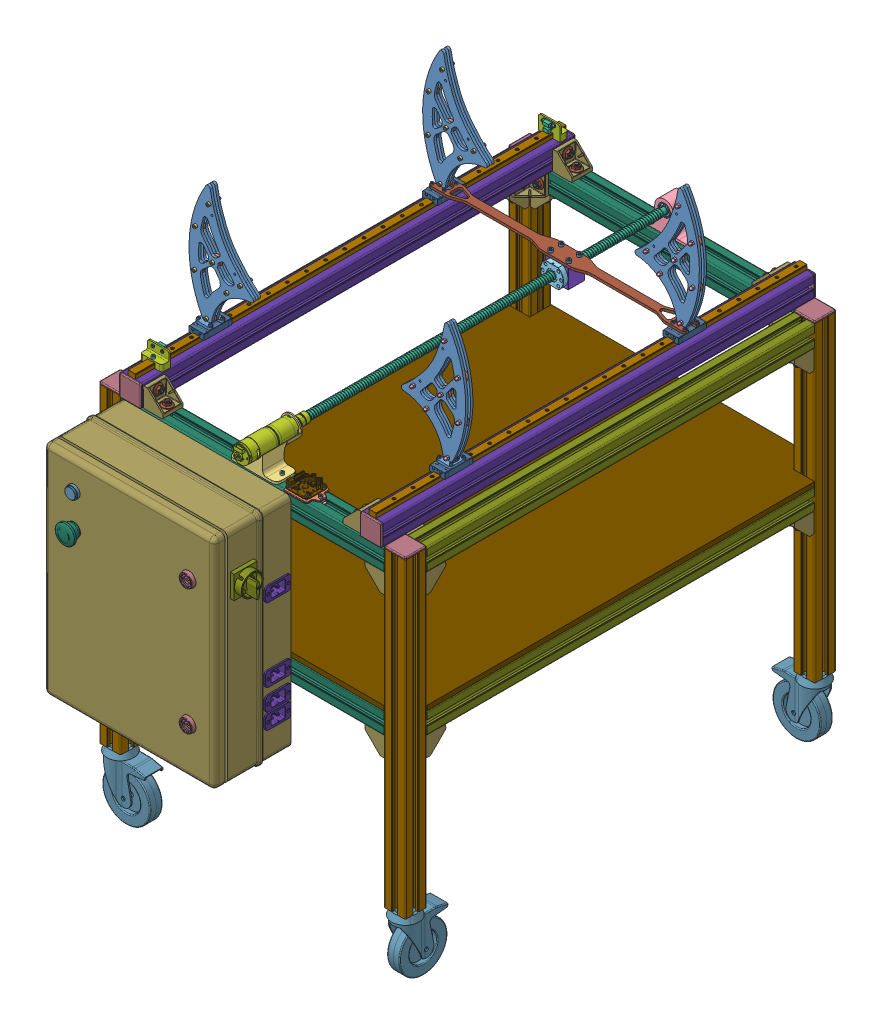
SolidWorks assembly Montaje_Eje_Z, configuration Predeterminado. Lengths in mm. (continued)
Components (placement in the parent): (continued)
- Montaje_Mesa.CATProduct-1: Montaje_Mesa.CATProduct [Predeterminado] at (176.75 -638.9678 608.5583) x (1 0 0) z (0 1 0) size (651 911 824) (continued)
  - Montaje_Escuadra.CATProduct-9: Montaje_Escuadra.CATProduct [Predeterminado] at (-398.921 484.3711 265.4998) x (-1 0 0) z (0 -1 0) size (52 42 52)
    - Tornillo_M8_Martillo.CATPart-1: Tornillo_M8_Martillo.CATPart [Predeterminado] at (0.029 0 50.8715) size (8.5 19 30)
    - Tuerca_M8.CATPart-1: Tuerca_M8.CATPart [Predeterminado] at (0.029 0 66.3715) size (21 21 8)
    - Bracket_45_B-Type_slot_10.CATPart-1: Bracket_45_B-Type_slot_10.CATPart [Predeterminado] at (29.279 0 56.8715) x (0 1 0) z (0 0 1) size (42 44.89 44.89)
    - Tuerca_M8.CATPart-2: Tuerca_M8.CATPart [Predeterminado] at (19.779 0 86.1215) x (0 0 1) z (-1 0 0) size (21 21 8)
    - Tornillo_M8_Martillo.CATPart-2: Tornillo_M8_Martillo.CATPart [Predeterminado] at (35.279 0 86.1215) x (0 0 1) z (-1 0 0) size (8.5 19 30)
  - Montaje_Escuadra.CATProduct-10: Montaje_Escuadra.CATProduct [Predeterminado] at (178.6715 501.7788 265.4998) x (0 -1 0) z (-1 0 0) size (52 42 52)
    - Tornillo_M8_Martillo.CATPart-1: Tornillo_M8_Martillo.CATPart [Predeterminado] at (0.029 0 50.8715) size (8.5 19 30)
    - Tuerca_M8.CATPart-1: Tuerca_M8.CATPart [Predeterminado] at (0.029 0 66.3715) size (21 21 8)
    - Bracket_45_B-Type_slot_10.CATPart-1: Bracket_45_B-Type_slot_10.CATPart [Predeterminado] at (29.279 0 56.8715) x (0 1 0) z (0 0 1) size (42 44.89 44.89)
    - Tuerca_M8.CATPart-2: Tuerca_M8.CATPart [Predeterminado] at (19.779 0 86.1215) x (0 0 1) z (-1 0 0) size (21 21 8)
    - Tornillo_M8_Martillo.CATPart-2: Tornillo_M8_Martillo.CATPart [Predeterminado] at (35.279 0 86.1215) x (0 0 1) z (-1 0 0) size (8.5 19 30)
  - Tabla_Inferior.CATPart-1: Tabla_Inferior.CATPart [Predeterminado] at (-153.2002 450 287.9998) x (1 0 0) z (0 0 1) size (640 900 10)
- Montaje_Pata_Robot-1: Montaje_Pata_Robot [Predeterminado] at (23.6979 293.1537 441.5005) x (1 -0.000086 0) z (0.000086 1 0) size (134.58 27 251.54)
  - Montaje_Pata_Robot.CATProduct-1: Montaje_Pata_Robot.CATProduct [Predeterminado] at origin size (134.58 27 251.54)
    - Pata_Ext.CATPart-1: Pata_Ext.CATPart [Predeterminado] at origin size (134.58 5 251.54)
    - Pata_Inter.CATPart-1: Pata_Inter.CATPart [Predeterminado] at (276.3973 -5 -199.417) x (0 1 0) z (0 0 1) size (5 20 20)
    - Pata_Inter.CATPart-2: Pata_Inter.CATPart [Predeterminado] at (251.6714 -5 -275.5) x (0 1 0) z (0 0 1) size (5 20 20)
    - Pata_Inter.CATPart-3: Pata_Inter.CATPart [Predeterminado] at (238.8294 -5 -167.7098) x (0 1 0) z (0 0 1) size (5 20 20)
    - Pata_Inter.CATPart-4: Pata_Inter.CATPart [Predeterminado] at (274.7433 -5 -119.4341) x (0 1 0) z (0 0 1) size (5 20 20)
    - Pata_Inter.CATPart-5: Pata_Inter.CATPart [Predeterminado] at (208.9667 -5 -207.8516) x (0 1 0) z (0 0 1) size (5 20 20)
    - Pata_Ext.CATPart-2: Pata_Ext.CATPart [Predeterminado] at (0 -10 0) size (134.58 5 251.54)
    - Tuerca_Tornillo.CATProduct-1: Tuerca_Tornillo.CATProduct [Predeterminado] at (180.6658 5 -180.6658) x (0 1 0) z (0 0 1) size (27 8.85 9.62)
      - ISO_4762_M4x20_STEEL_HEXAGON_SOCKET_HEAD_CAP_SCREW.CATPart-1: ISO_4762_M4x20_STEEL_HEXAGON_SOCKET_HEAD_CAP_SCREW.CATPart [Predeterminado] at origin size (24 7 7)
      - 1587_M4_Tuerca_Ciega.CATPart-1: 1587_M4_Tuerca_Ciega.CATPart [Predeterminado] at (-15 0 0) x (-1 0 0) z (0 0.965909 -0.258881) size (8 8.08 7)
    - Tuerca_Tornillo.CATProduct-2: Tuerca_Tornillo.CATProduct [Predeterminado] at (276.3973 5 -199.417) x (0 1 0) z (0 0 1) size (27 8.85 9.62)
      - ISO_4762_M4x20_STEEL_HEXAGON_SOCKET_HEAD_CAP_SCREW.CATPart-1: ISO_4762_M4x20_STEEL_HEXAGON_SOCKET_HEAD_CAP_SCREW.CATPart [Predeterminado] at origin size (24 7 7)
      - 1587_M4_Tuerca_Ciega.CATPart-1: 1587_M4_Tuerca_Ciega.CATPart [Predeterminado] at (-15 0 0) x (-1 0 0) z (0 0.965909 -0.258881) size (8 8.08 7)
    - Tuerca_Tornillo.CATProduct-3: Tuerca_Tornillo.CATProduct [Predeterminado] at (238.8294 5 -167.7098) x (0 1 0) z (0 0 1) size (27 8.85 9.62)
      - ISO_4762_M4x20_STEEL_HEXAGON_SOCKET_HEAD_CAP_SCREW.CATPart-1: ISO_4762_M4x20_STEEL_HEXAGON_SOCKET_HEAD_CAP_SCREW.CATPart [Predeterminado] at origin size (24 7 7)
      - 1587_M4_Tuerca_Ciega.CATPart-1: 1587_M4_Tuerca_Ciega.CATPart [Predeterminado] at (-15 0 0) x (-1 0 0) z (0 0.965909 -0.258881) size (8 8.08 7)
    - Tuerca_Tornillo.CATProduct-4: Tuerca_Tornillo.CATProduct [Predeterminado] at (251.6714 5 -275.5) x (0 1 0) z (0 0 1) size (27 8.85 9.62)
      - ISO_4762_M4x20_STEEL_HEXAGON_SOCKET_HEAD_CAP_SCREW.CATPart-1: ISO_4762_M4x20_STEEL_HEXAGON_SOCKET_HEAD_CAP_SCREW.CATPart [Predeterminado] at origin size (24 7 7)
      - 1587_M4_Tuerca_Ciega.CATPart-1: 1587_M4_Tuerca_Ciega.CATPart [Predeterminado] at (-15 0 0) x (-1 0 0) z (0 0.965909 -0.258881) size (8 8.08 7)
    - Tuerca_Tornillo.CATProduct-5: Tuerca_Tornillo.CATProduct [Predeterminado] at (274.7433 5 -119.4341) x (0 1 0) z (0 0 1) size (27 8.85 9.62)
      - ISO_4762_M4x20_STEEL_HEXAGON_SOCKET_HEAD_CAP_SCREW.CATPart-1: ISO_4762_M4x20_STEEL_HEXAGON_SOCKET_HEAD_CAP_SCREW.CATPart [Predeterminado] at origin size (24 7 7)
      - 1587_M4_Tuerca_Ciega.CATPart-1: 1587_M4_Tuerca_Ciega.CATPart [Predeterminado] at (-15 0 0) x (-1 0 0) z (0 0.965909 -0.258881) size (8 8.08 7)
    - Tuerca_Tornillo.CATProduct-6: Tuerca_Tornillo.CATProduct [Predeterminado] at (246.794 5 -66.1283) x (0 1 0) z (0 0 1) size (27 8.85 9.62)
      - ISO_4762_M4x20_STEEL_HEXAGON_SOCKET_HEAD_CAP_SCREW.CATPart-1: ISO_4762_M4x20_STEEL_HEXAGON_SOCKET_HEAD_CAP_SCREW.CATPart [Predeterminado] at origin size (24 7 7)
      - 1587_M4_Tuerca_Ciega.CATPart-1: 1587_M4_Tuerca_Ciega.CATPart [Predeterminado] at (-15 0 0) x (-1 0 0) z (0 0.965909 -0.258881) size (8 8.08 7)
    - Tuerca_Tornillo.CATProduct-7: Tuerca_Tornillo.CATProduct [Predeterminado] at (208.9667 5 -207.8516) x (0 1 0) z (0 0 1) size (27 8.85 9.62)
      - ISO_4762_M4x20_STEEL_HEXAGON_SOCKET_HEAD_CAP_SCREW.CATPart-1: ISO_4762_M4x20_STEEL_HEXAGON_SOCKET_HEAD_CAP_SCREW.CATPart [Predeterminado] at origin size (24 7 7)
      - 1587_M4_Tuerca_Ciega.CATPart-1: 1587_M4_Tuerca_Ciega.CATPart [Predeterminado] at (-15 0 0) x (-1 0 0) z (0 0.965909 -0.258881) size (8 8.08 7)
- Montaje_Pata_Robot.CATProduct-1: Montaje_Pata_Robot.CATProduct [Predeterminado] at (23.6979 293.1537 -46.4995) x (1 -0.000086 0) z (0.000086 1 0) size (134.58 27 251.54)
  - Pata_Ext.CATPart-1: Pata_Ext.CATPart [Predeterminado] at origin size (134.58 5 251.54)
  - Pata_Inter.CATPart-1: Pata_Inter.CATPart [Predeterminado] at (276.3973 -5 -199.417) x (0 1 0) z (0 0 1) size (5 20 20)
  - Pata_Inter.CATPart-2: Pata_Inter.CATPart [Predeterminado] at (251.6714 -5 -275.5) x (0 1 0) z (0 0 1) size (5 20 20)
  - Pata_Inter.CATPart-3: Pata_Inter.CATPart [Predeterminado] at (238.8294 -5 -167.7098) x (0 1 0) z (0 0 1) size (5 20 20)
  - Pata_Inter.CATPart-4: Pata_Inter.CATPart [Predeterminado] at (274.7433 -5 -119.4341) x (0 1 0) z (0 0 1) size (5 20 20)
  - Pata_Inter.CATPart-5: Pata_Inter.CATPart [Predeterminado] at (208.9667 -5 -207.8516) x (0 1 0) z (0 0 1) size (5 20 20)
  - Pata_Ext.CATPart-2: Pata_Ext.CATPart [Predeterminado] at (0 -10 0) size (134.58 5 251.54)
  - Tuerca_Tornillo.CATProduct-1: Tuerca_Tornillo.CATProduct [Predeterminado] at (180.6658 5 -180.6658) x (0 1 0) z (0 0 1) size (27 8.85 9.62)
    - ISO_4762_M4x20_STEEL_HEXAGON_SOCKET_HEAD_CAP_SCREW.CATPart-1: ISO_4762_M4x20_STEEL_HEXAGON_SOCKET_HEAD_CAP_SCREW.CATPart [Predeterminado] at origin size (24 7 7)
    - 1587_M4_Tuerca_Ciega.CATPart-1: 1587_M4_Tuerca_Ciega.CATPart [Predeterminado] at (-15 0 0) x (-1 0 0) z (0 0.965909 -0.258881) size (8 8.08 7)
  - Tuerca_Tornillo.CATProduct-2: Tuerca_Tornillo.CATProduct [Predeterminado] at (276.3973 5 -199.417) x (0 1 0) z (0 0 1) size (27 8.85 9.62)
    - ISO_4762_M4x20_STEEL_HEXAGON_SOCKET_HEAD_CAP_SCREW.CATPart-1: ISO_4762_M4x20_STEEL_HEXAGON_SOCKET_HEAD_CAP_SCREW.CATPart [Predeterminado] at origin size (24 7 7)
    - 1587_M4_Tuerca_Ciega.CATPart-1: 1587_M4_Tuerca_Ciega.CATPart [Predeterminado] at (-15 0 0) x (-1 0 0) z (0 0.965909 -0.258881) size (8 8.08 7)
  - Tuerca_Tornillo.CATProduct-3: Tuerca_Tornillo.CATProduct [Predeterminado] at (238.8294 5 -167.7098) x (0 1 0) z (0 0 1) size (27 8.85 9.62)
    - ISO_4762_M4x20_STEEL_HEXAGON_SOCKET_HEAD_CAP_SCREW.CATPart-1: ISO_4762_M4x20_STEEL_HEXAGON_SOCKET_HEAD_CAP_SCREW.CATPart [Predeterminado] at origin size (24 7 7)
    - 1587_M4_Tuerca_Ciega.CATPart-1: 1587_M4_Tuerca_Ciega.CATPart [Predeterminado] at (-15 0 0) x (-1 0 0) z (0 0.965909 -0.258881) size (8 8.08 7)
  - Tuerca_Tornillo.CATProduct-4: Tuerca_Tornillo.CATProduct [Predeterminado] at (251.6714 5 -275.5) x (0 1 0) z (0 0 1) size (27 8.85 9.62)
    - ISO_4762_M4x20_STEEL_HEXAGON_SOCKET_HEAD_CAP_SCREW.CATPart-1: ISO_4762_M4x20_STEEL_HEXAGON_SOCKET_HEAD_CAP_SCREW.CATPart [Predeterminado] at origin size (24 7 7)
    - 1587_M4_Tuerca_Ciega.CATPart-1: 1587_M4_Tuerca_Ciega.CATPart [Predeterminado] at (-15 0 0) x (-1 0 0) z (0 0.965909 -0.258881) size (8 8.08 7)
  - Tuerca_Tornillo.CATProduct-5: Tuerca_Tornillo.CATProduct [Predeterminado] at (274.7433 5 -119.4341) x (0 1 0) z (0 0 1) size (27 8.85 9.62)
    - ISO_4762_M4x20_STEEL_HEXAGON_SOCKET_HEAD_CAP_SCREW.CATPart-1: ISO_4762_M4x20_STEEL_HEXAGON_SOCKET_HEAD_CAP_SCREW.CATPart [Predeterminado] at origin size (24 7 7)
    - 1587_M4_Tuerca_Ciega.CATPart-1: 1587_M4_Tuerca_Ciega.CATPart [Predeterminado] at (-15 0 0) x (-1 0 0) z (0 0.965909 -0.258881) size (8 8.08 7)
  - Tuerca_Tornillo.CATProduct-6: Tuerca_Tornillo.CATProduct [Predeterminado] at (246.794 5 -66.1283) x (0 1 0) z (0 0 1) size (27 8.85 9.62)
    - ISO_4762_M4x20_STEEL_HEXAGON_SOCKET_HEAD_CAP_SCREW.CATPart-1: ISO_4762_M4x20_STEEL_HEXAGON_SOCKET_HEAD_CAP_SCREW.CATPart [Predeterminado] at origin size (24 7 7)
    - 1587_M4_Tuerca_Ciega.CATPart-1: 1587_M4_Tuerca_Ciega.CATPart [Predeterminado] at (-15 0 0) x (-1 0 0) z (0 0.965909 -0.258881) size (8 8.08 7)
  - Tuerca_Tornillo.CATProduct-7: Tuerca_Tornillo.CATProduct [Predeterminado] at (208.9667 5 -207.8516) x (0 1 0) z (0 0 1) size (27 8.85 9.62)
    - ISO_4762_M4x20_STEEL_HEXAGON_SOCKET_HEAD_CAP_SCREW.CATPart-1: ISO_4762_M4x20_STEEL_HEXAGON_SOCKET_HEAD_CAP_SCREW.CATPart [Predeterminado] at origin size (24 7 7)
    - 1587_M4_Tuerca_Ciega.CATPart-1: 1587_M4_Tuerca_Ciega.CATPart [Predeterminado] at (-15 0 0) x (-1 0 0) z (0 0.965909 -0.258881) size (8 8.08 7)
- Montaje_Pata_Robot.CATProduct-2: Montaje_Pata_Robot.CATProduct [Predeterminado] at (23.6979 293.1537 446.5005) x (-1 -0.000085 0) z (-0.000085 1 0) size (134.58 27 251.54)
  - Pata_Ext.CATPart-1: Pata_Ext.CATPart [Predeterminado] at origin size (134.58 5 251.54)
  - Pata_Inter.CATPart-1: Pata_Inter.CATPart [Predeterminado] at (276.3973 -5 -199.417) x (0 1 0) z (0 0 1) size (5 20 20)
  - Pata_Inter.CATPart-2: Pata_Inter.CATPart [Predeterminado] at (251.6714 -5 -275.5) x (0 1 0) z (0 0 1) size (5 20 20)
  - Pata_Inter.CATPart-3: Pata_Inter.CATPart [Predeterminado] at (238.8294 -5 -167.7098) x (0 1 0) z (0 0 1) size (5 20 20)
  - Pata_Inter.CATPart-4: Pata_Inter.CATPart [Predeterminado] at (274.7433 -5 -119.4341) x (0 1 0) z (0 0 1) size (5 20 20)
  - Pata_Inter.CATPart-5: Pata_Inter.CATPart [Predeterminado] at (208.9667 -5 -207.8516) x (0 1 0) z (0 0 1) size (5 20 20)
  - Pata_Ext.CATPart-2: Pata_Ext.CATPart [Predeterminado] at (0 -10 0) size (134.58 5 251.54)
  - Tuerca_Tornillo.CATProduct-1: Tuerca_Tornillo.CATProduct [Predeterminado] at (180.6658 5 -180.6658) x (0 1 0) z (0 0 1) size (27 8.85 9.62)
    - ISO_4762_M4x20_STEEL_HEXAGON_SOCKET_HEAD_CAP_SCREW.CATPart-1: ISO_4762_M4x20_STEEL_HEXAGON_SOCKET_HEAD_CAP_SCREW.CATPart [Predeterminado] at origin size (24 7 7)
    - 1587_M4_Tuerca_Ciega.CATPart-1: 1587_M4_Tuerca_Ciega.CATPart [Predeterminado] at (-15 0 0) x (-1 0 0) z (0 0.965909 -0.258881) size (8 8.08 7)
  - Tuerca_Tornillo.CATProduct-2: Tuerca_Tornillo.CATProduct [Predeterminado] at (276.3973 5 -199.417) x (0 1 0) z (0 0 1) size (27 8.85 9.62)
    - ISO_4762_M4x20_STEEL_HEXAGON_SOCKET_HEAD_CAP_SCREW.CATPart-1: ISO_4762_M4x20_STEEL_HEXAGON_SOCKET_HEAD_CAP_SCREW.CATPart [Predeterminado] at origin size (24 7 7)
    - 1587_M4_Tuerca_Ciega.CATPart-1: 1587_M4_Tuerca_Ciega.CATPart [Predeterminado] at (-15 0 0) x (-1 0 0) z (0 0.965909 -0.258881) size (8 8.08 7)
  - Tuerca_Tornillo.CATProduct-3: Tuerca_Tornillo.CATProduct [Predeterminado] at (238.8294 5 -167.7098) x (0 1 0) z (0 0 1) size (27 8.85 9.62)
    - ISO_4762_M4x20_STEEL_HEXAGON_SOCKET_HEAD_CAP_SCREW.CATPart-1: ISO_4762_M4x20_STEEL_HEXAGON_SOCKET_HEAD_CAP_SCREW.CATPart [Predeterminado] at origin size (24 7 7)
    - 1587_M4_Tuerca_Ciega.CATPart-1: 1587_M4_Tuerca_Ciega.CATPart [Predeterminado] at (-15 0 0) x (-1 0 0) z (0 0.965909 -0.258881) size (8 8.08 7)
  - Tuerca_Tornillo.CATProduct-4: Tuerca_Tornillo.CATProduct [Predeterminado] at (251.6714 5 -275.5) x (0 1 0) z (0 0 1) size (27 8.85 9.62)
    - ISO_4762_M4x20_STEEL_HEXAGON_SOCKET_HEAD_CAP_SCREW.CATPart-1: ISO_4762_M4x20_STEEL_HEXAGON_SOCKET_HEAD_CAP_SCREW.CATPart [Predeterminado] at origin size (24 7 7)
    - 1587_M4_Tuerca_Ciega.CATPart-1: 1587_M4_Tuerca_Ciega.CATPart [Predeterminado] at (-15 0 0) x (-1 0 0) z (0 0.965909 -0.258881) size (8 8.08 7)
  - Tuerca_Tornillo.CATProduct-5: Tuerca_Tornillo.CATProduct [Predeterminado] at (274.7433 5 -119.4341) x (0 1 0) z (0 0 1) size (27 8.85 9.62)
    - ISO_4762_M4x20_STEEL_HEXAGON_SOCKET_HEAD_CAP_SCREW.CATPart-1: ISO_4762_M4x20_STEEL_HEXAGON_SOCKET_HEAD_CAP_SCREW.CATPart [Predeterminado] at origin size (24 7 7)
    - 1587_M4_Tuerca_Ciega.CATPart-1: 1587_M4_Tuerca_Ciega.CATPart [Predeterminado] at (-15 0 0) x (-1 0 0) z (0 0.965909 -0.258881) size (8 8.08 7)
  - Tuerca_Tornillo.CATProduct-6: Tuerca_Tornillo.CATProduct [Predeterminado] at (246.794 5 -66.1283) x (0 1 0) z (0 0 1) size (27 8.85 9.62)
    - ISO_4762_M4x20_STEEL_HEXAGON_SOCKET_HEAD_CAP_SCREW.CATPart-1: ISO_4762_M4x20_STEEL_HEXAGON_SOCKET_HEAD_CAP_SCREW.CATPart [Predeterminado] at origin size (24 7 7)
    - 1587_M4_Tuerca_Ciega.CATPart-1: 1587_M4_Tuerca_Ciega.CATPart [Predeterminado] at (-15 0 0) x (-1 0 0) z (0 0.965909 -0.258881) size (8 8.08 7)
  - Tuerca_Tornillo.CATProduct-7: Tuerca_Tornillo.CATProduct [Predeterminado] at (208.9667 5 -207.8516) x (0 1 0) z (0 0 1) size (27 8.85 9.62)
    - ISO_4762_M4x20_STEEL_HEXAGON_SOCKET_HEAD_CAP_SCREW.CATPart-1: ISO_4762_M4x20_STEEL_HEXAGON_SOCKET_HEAD_CAP_SCREW.CATPart [Predeterminado] at origin size (24 7 7)
    - 1587_M4_Tuerca_Ciega.CATPart-1: 1587_M4_Tuerca_Ciega.CATPart [Predeterminado] at (-15 0 0) x (-1 0 0) z (0 0.965909 -0.258881) size (8 8.08 7)
- Montaje_Pata_Robot.CATProduct-3: Montaje_Pata_Robot.CATProduct [Predeterminado] at (23.6979 293.1537 -41.4995) x (-1 -0.000085 0) z (-0.000085 1 0) size (134.58 27 251.54)
  - Pata_Ext.CATPart-1: Pata_Ext.CATPart [Predeterminado] at origin size (134.58 5 251.54)
  - Pata_Inter.CATPart-1: Pata_Inter.CATPart [Predeterminado] at (276.3973 -5 -199.417) x (0 1 0) z (0 0 1) size (5 20 20)
  - Pata_Inter.CATPart-2: Pata_Inter.CATPart [Predeterminado] at (251.6714 -5 -275.5) x (0 1 0) z (0 0 1) size (5 20 20)
  - Pata_Inter.CATPart-3: Pata_Inter.CATPart [Predeterminado] at (238.8294 -5 -167.7098) x (0 1 0) z (0 0 1) size (5 20 20)
  - Pata_Inter.CATPart-4: Pata_Inter.CATPart [Predeterminado] at (274.7433 -5 -119.4341) x (0 1 0) z (0 0 1) size (5 20 20)
  - Pata_Inter.CATPart-5: Pata_Inter.CATPart [Predeterminado] at (208.9667 -5 -207.8516) x (0 1 0) z (0 0 1) size (5 20 20)
  - Pata_Ext.CATPart-2: Pata_Ext.CATPart [Predeterminado] at (0 -10 0) size (134.58 5 251.54)
  - Tuerca_Tornillo.CATProduct-1: Tuerca_Tornillo.CATProduct [Predeterminado] at (180.6658 5 -180.6658) x (0 1 0) z (0 0 1) size (27 8.85 9.62)
    - ISO_4762_M4x20_STEEL_HEXAGON_SOCKET_HEAD_CAP_SCREW.CATPart-1: ISO_4762_M4x20_STEEL_HEXAGON_SOCKET_HEAD_CAP_SCREW.CATPart [Predeterminado] at origin size (24 7 7)
    - 1587_M4_Tuerca_Ciega.CATPart-1: 1587_M4_Tuerca_Ciega.CATPart [Predeterminado] at (-15 0 0) x (-1 0 0) z (0 0.965909 -0.258881) size (8 8.08 7)
  - Tuerca_Tornillo.CATProduct-2: Tuerca_Tornillo.CATProduct [Predeterminado] at (276.3973 5 -199.417) x (0 1 0) z (0 0 1) size (27 8.85 9.62)
    - ISO_4762_M4x20_STEEL_HEXAGON_SOCKET_HEAD_CAP_SCREW.CATPart-1: ISO_4762_M4x20_STEEL_HEXAGON_SOCKET_HEAD_CAP_SCREW.CATPart [Predeterminado] at origin size (24 7 7)
    - 1587_M4_Tuerca_Ciega.CATPart-1: 1587_M4_Tuerca_Ciega.CATPart [Predeterminado] at (-15 0 0) x (-1 0 0) z (0 0.965909 -0.258881) size (8 8.08 7)
  - Tuerca_Tornillo.CATProduct-3: Tuerca_Tornillo.CATProduct [Predeterminado] at (238.8294 5 -167.7098) x (0 1 0) z (0 0 1) size (27 8.85 9.62)
    - ISO_4762_M4x20_STEEL_HEXAGON_SOCKET_HEAD_CAP_SCREW.CATPart-1: ISO_4762_M4x20_STEEL_HEXAGON_SOCKET_HEAD_CAP_SCREW.CATPart [Predeterminado] at origin size (24 7 7)
    - 1587_M4_Tuerca_Ciega.CATPart-1: 1587_M4_Tuerca_Ciega.CATPart [Predeterminado] at (-15 0 0) x (-1 0 0) z (0 0.965909 -0.258881) size (8 8.08 7)
  - Tuerca_Tornillo.CATProduct-4: Tuerca_Tornillo.CATProduct [Predeterminado] at (251.6714 5 -275.5) x (0 1 0) z (0 0 1) size (27 8.85 9.62)
    - ISO_4762_M4x20_STEEL_HEXAGON_SOCKET_HEAD_CAP_SCREW.CATPart-1: ISO_4762_M4x20_STEEL_HEXAGON_SOCKET_HEAD_CAP_SCREW.CATPart [Predeterminado] at origin size (24 7 7)
    - 1587_M4_Tuerca_Ciega.CATPart-1: 1587_M4_Tuerca_Ciega.CATPart [Predeterminado] at (-15 0 0) x (-1 0 0) z (0 0.965909 -0.258881) size (8 8.08 7)
  - Tuerca_Tornillo.CATProduct-5: Tuerca_Tornillo.CATProduct [Predeterminado] at (274.7433 5 -119.4341) x (0 1 0) z (0 0 1) size (27 8.85 9.62)
    - ISO_4762_M4x20_STEEL_HEXAGON_SOCKET_HEAD_CAP_SCREW.CATPart-1: ISO_4762_M4x20_STEEL_HEXAGON_SOCKET_HEAD_CAP_SCREW.CATPart [Predeterminado] at origin size (24 7 7)
    - 1587_M4_Tuerca_Ciega.CATPart-1: 1587_M4_Tuerca_Ciega.CATPart [Predeterminado] at (-15 0 0) x (-1 0 0) z (0 0.965909 -0.258881) size (8 8.08 7)
  - Tuerca_Tornillo.CATProduct-6: Tuerca_Tornillo.CATProduct [Predeterminado] at (246.794 5 -66.1283) x (0 1 0) z (0 0 1) size (27 8.85 9.62)
    - ISO_4762_M4x20_STEEL_HEXAGON_SOCKET_HEAD_CAP_SCREW.CATPart-1: ISO_4762_M4x20_STEEL_HEXAGON_SOCKET_HEAD_CAP_SCREW.CATPart [Predeterminado] at origin size (24 7 7)
    - 1587_M4_Tuerca_Ciega.CATPart-1: 1587_M4_Tuerca_Ciega.CATPart [Predeterminado] at (-15 0 0) x (-1 0 0) z (0 0.965909 -0.258881) size (8 8.08 7)
  - Tuerca_Tornillo.CATProduct-7: Tuerca_Tornillo.CATProduct [Predeterminado] at (208.9667 5 -207.8516) x (0 1 0) z (0 0 1) size (27 8.85 9.62)
    - ISO_4762_M4x20_STEEL_HEXAGON_SOCKET_HEAD_CAP_SCREW.CATPart-1: ISO_4762_M4x20_STEEL_HEXAGON_SOCKET_HEAD_CAP_SCREW.CATPart [Predeterminado] at origin size (24 7 7)
    - 1587_M4_Tuerca_Ciega.CATPart-1: 1587_M4_Tuerca_Ciega.CATPart [Predeterminado] at (-15 0 0) x (-1 0 0) z (0 0.965909 -0.258881) size (8 8.08 7)
- SFU1605-1: SFU1605 [По умолчанию] at (24.5502 -12.1678 -66.4995) x (0 1 0) z (0 0 1) size (40 48 50)
- SCR1605-Z-1: SCR1605-Z [850mm] at (24.5502 -12.1678 -292.8415) x (-0.848768 0.528765 0) z (-0.528765 -0.848768 0) size (16.45 800 18.52)
- Flexible_Coupling_8x8.CATPart-1: Flexible_Coupling_8x8.CATPart [Predeterminado] at (24.5502 -12.1678 545.4741) x (0.984327 -0.176353 0) z (-0.176353 -0.984327 0) size (20 30.8 20)
- HD16-1: HD16 [Default] at (24.5502 7.8322 -26.4995) x (-1 0 0) z (0 0 -1) size (48 40 35)
- MGN15 rail-2: MGN15 rail [MGN15] at (275.0502 -5.9678 -291.2916) x (1 0 0) z (0 0 1) size (15 10 900)
- MGN15C-1: MGN15C [MGN15C] at (275.0502 1.8322 444.0005) x (1 0 0) z (0 0 1) size (32 12 61.91)
- MGN15 rail-3: MGN15 rail [MGN15] at (-227.9501 -5.9677 -291.5915) x (1 0 0) z (0 0 1) size (15 10 900)
- MGN15C-2: MGN15C [MGN15C] at (275.0502 1.8322 -43.9995) x (1 0 0) z (0 0 1) size (32 12 61.91)
- MGN15C-3: MGN15C [MGN15C] at (-227.9501 1.8323 -43.9995) x (1 0 0) z (0 0 1) size (32 12 61.91)
- MGN15C-4: MGN15C [MGN15C] at (-227.9501 1.8323 444.0005) x (1 0 0) z (0 0 1) size (32 12 61.91)
- Viga_Union-1: Viga_Union [Predeterminado] at (23.5502 7.8322 -43.9995) x (1 0 0) z (0 0 1) size (535 5 35)
- Armario-1: Armario [Predeterminado] at (-73.45 -286.9678 608.5586) x (1 0 0) z (0 0 1) size (393.04 462 183.02)
  - Caja-1: Caja [Predeterminado] at origin size (362 462 160)
  - Cerradura-1: Cerradura [Predeterminado] at (124.7293 131.0942 160) x (-1 0 0) z (0 0 -1) size (30 30 7)
  - Cerradura-2: Cerradura [Predeterminado] at (124.7293 -131.0942 160) x (-1 0 0) z (0 0 -1) size (30 30 7)
  - LED Status -G-2: LED Status -G [Default] at (-114.8478 170.1961 160) x (1 0 0) z (0 -1 0) size (25 8.7 25)
  - E-Stop Button [ZB4BS844]-1: E-Stop Button [ZB4BS844] [Default] at (-114.8768 101.0908 175) x (1 0 0) z (0 -1 0) size (40.81 55.91 40.81)
  - Lovato GX15 690V 16A Isolator Switch Model-1: Lovato GX15 690V 16A Isolator Switch Model [Default] at (125 129.4942 102.5) x (0 0 -1) z (0 -1 0) size (48 87.04 48)
  - Einbau-Gerätestecker 24V_16A.step-3: Einbau-Gerätestecker 24V_16A.step [Predeterminado] at (178 -121.6068 29.3038) x (0 0 -1) z (1 0 0) size (53 30 31.6)
  - Einbau-Gerätestecker 24V_16A.step-2: Einbau-Gerätestecker 24V_16A.step [Predeterminado] at (178 76.4158 29.3038) x (0 0 -1) z (1 0 0) size (53 30 31.6)
  - Einbau-Gerätestecker 24V_16A.step-4: Einbau-Gerätestecker 24V_16A.step [Predeterminado] at (178 -154.4225 29.3038) x (0 0 -1) z (1 0 0) size (53 30 31.6)
  - Einbau-Gerätestecker 24V_16A.step-5: Einbau-Gerätestecker 24V_16A.step [Predeterminado] at (178 -76.9075 29.3038) x (0 0 -1) z (1 0 0) size (53 30 31.6)
- PCB_Control_Motores_V2.catpart-1: PCB_Control_Motores_V2.catpart [Predeterminado] at (30.5531 -47.9293 524.0575) x (0 0 1) z (0 1 0) size (48 50.39 14.79)
- Sujección-1: Sujección [Predeterminado] at (275.0502 7.8322 444.0005) x (1 0 0) z (0 0 1) size (31.99 5 35)
- Sujección-2: Sujección [Predeterminado] at (-227.9501 7.8323 444.0005) x (-1 0 0) z (0 0 -1) size (31.99 5 35)
- Soporte_PCB_Motor_Z-1: Soporte_PCB_Motor_Z [Predeterminado] at (114.6751 -55.9678 585.7153) x (1 0 0) z (0 0 1) size (70 3 50)
- Soporte_Motor_Eje_Z-1: Soporte_Motor_Eje_Z [Predeterminado] at (24.5502 -53.4678 563.5585) x (1 0 0) z (0 0 1) size (100 65.01 82.6)
- Soporte_Husillo_Eje_Z-1: Soporte_Husillo_Eje_Z [Predeterminado] at (24.5502 -53.4678 -286.4416) x (1 0 0) z (0 0 1) size (100 63.8 35)
- 6000-Bearing-1: 6000-Bearing [Default] at (24.5502 -12.1678 -259.4416) x (1 0 0) z (0 0 1) size (26 26 8)
- 6000-Bearing-2: 6000-Bearing [Default] at (24.5502 -12.1678 -286.4416) x (1 0 0) z (0 0 1) size (26 26 8)
- End_Stop-1: End_Stop [Predeterminado] at (-227.9501 14.0323 550.4085) x (-1 0 0) z (0 0 -1) size (27 18 10.1)
- End_Stop-2: End_Stop [Predeterminado] at (-227.9501 14.0323 -263.5915) x (1 0 0) z (0 0 1) size (27 18 10.1)
- Soporte_FdC_Eje_Z-1: Soporte_FdC_Eje_Z [Predeterminado] at (-205.4501 0.5323 -272.5915) x (-1 0 0) z (0 0 -1) size (45 31 18)
- Soporte_FdC_Eje_Z-2: Soporte_FdC_Eje_Z [Predeterminado] at (-250.4501 0.5323 559.4085) x (1 0 0) z (0 0 1) size (45 31 18)
Mates (geometry in assembly coordinates):
- Concéntrica2: concentric aligned: circle of Montaje_Pata_Robot.CATProduct-2/Pata_Ext.CATPart-2; circle of Montaje_Pata_Robot.CATProduct-3/Pata_Ext.CATPart-2
- Concéntrica3: concentric aligned: circle of Montaje_Pata_Robot-1/Montaje_Pata_Robot.CATProduct-1/Pata_Ext.CATPart-1; circle of Montaje_Pata_Robot.CATProduct-1/Pata_Ext.CATPart-1
- Distancia1: distance = 473 mm anti-aligned: plane of Montaje_Pata_Robot.CATProduct-2/Pata_Ext.CATPart-2 through (23.6979 293.1537 436.5005) normal (0 0 -1); plane of Montaje_Pata_Robot.CATProduct-3/Pata_Ext.CATPart-1 through (23.6979 293.1537 -36.4995) normal (0 0 1)
- Distancia2: distance = 473 mm anti-aligned: plane of Montaje_Pata_Robot-1/Montaje_Pata_Robot.CATProduct-1/Pata_Ext.CATPart-1 through (23.6979 293.1537 436.5005) normal (0 0 -1); plane of Montaje_Pata_Robot.CATProduct-1/Pata_Ext.CATPart-2 through (23.6979 293.1537 -36.4995) normal (0 0 1)
- Coincidente7: coincident aligned: plane of Montaje_Pata_Robot.CATProduct-1/Pata_Ext.CATPart-1 through (23.6979 293.1537 -51.4995) normal (0 0 -1); plane of Montaje_Pata_Robot.CATProduct-3/Pata_Ext.CATPart-2 through (23.6979 293.1537 -51.4995) normal (0 0 -1)
- Coincidente17: coincident anti-aligned: plane of Motor_Tornillos-1/Motor_Tornillos.CATProduct-1/CHP-36GP-555.CATPart-1 through (24.5502 -12.1678 526.9585) normal (0 0 -1); plane of Flexible_Coupling_8x8.CATPart-1 through (24.5502 -12.1678 526.9585) normal (0 0 1)
- Concéntrica5: concentric aligned: circle of SCR1605-Z-1; circle of Flexible_Coupling_8x8.CATPart-1
- Coincidente18: coincident anti-aligned: plane of SCR1605-Z-1 through (31.3403 -16.398 496.1585) normal (0 0 1); plane of Flexible_Coupling_8x8.CATPart-1 through (24.5502 -12.1678 496.1585) normal (0 0 -1)
- Concéntrica6: concentric aligned: circle of SFU1605-1; circle of SCR1605-Z-1
- Coincidente21: coincident anti-aligned: plane of SFU1605-1 through (24.5502 -12.1678 -26.4995) normal (0 0 -1); plane of HD16-1 through (24.5502 -12.1678 -26.4995) normal (0 0 1)
- Concéntrica8: concentric anti-aligned: circle of SFU1605-1; circle of HD16-1
- Concéntrica9: concentric aligned: circle of SFU1605-1; circle of HD16-1
- Coincidente25: coincident anti-aligned: plane of Montaje_Mesa.CATProduct-1/Montaje_Carril.CATProduct-1/P45L_N10_B_900.CATPart-1 through (281.1501 -10.9677 -291.2916) normal (0 1 0); plane of MGN15 rail-2 through (267.7502 -10.9678 608.7084) normal (0 -1 0)
- Distancia8: distance = 15 mm aligned: plane of MGN15 rail-2 through (282.5502 -10.7678 608.7084) normal (1 0 0); plane of Montaje_Mesa.CATProduct-1/Montaje_Carril.CATProduct-1/P45L_N10_B_900.CATPart-1 through (297.5502 -39.5678 -291.2916) normal (1 0 0)
- Coincidente27: coincident anti-aligned: plane of Montaje_Mesa.CATProduct-1/Montaje_Carril.CATProduct-1/Tapa 45x45.CATPart-1 through (275.05 -33.4678 -291.2916) normal (0 0 1); plane of MGN15 rail-2 through (267.4502 -2.4678 -291.2916) normal (0 0 -1)
- Distancia10: distance = 15 mm aligned: plane of MGN15 rail-3 through (-235.4501 -10.7677 608.4085) normal (-1 0 0); plane of Montaje_Mesa.CATProduct-1/Montaje_Carril.CATProduct-2/P45L_N10_B_900.CATPart-1 through (-250.4501 -39.5678 608.4085) normal (-1 0 0)
- Coincidente32: coincident anti-aligned: plane of MGN15 rail-2 through (282.5502 -10.7678 608.7084) normal (1 0 0); plane of MGN15C-1 through (282.5502 1.8322 465.7005) normal (-1 0 0)
- Coincidente33: coincident anti-aligned: plane of MGN15 rail-2 through (267.7502 -0.9678 608.7084) normal (0 1 0); plane of MGN15C-1 through (275.0502 -0.9678 465.7005) normal (0 -1 0)
- Coincidente34: coincident anti-aligned: plane of MGN15 rail-2 through (267.7502 -0.9678 608.7084) normal (0 1 0); plane of MGN15C-2 through (275.0502 -0.9678 -22.2995) normal (0 -1 0)
- Coincidente35: coincident anti-aligned: plane of MGN15 rail-2 through (282.5502 -10.7678 608.7084) normal (1 0 0); plane of MGN15C-2 through (282.5502 1.8322 -72.4995) normal (-1 0 0)
- Distancia11: distance = 429.2 mm anti-aligned: plane of MGN15C-2 through (275.0502 1.8322 -14.5995) normal (0 0 1); plane of MGN15C-1 through (275.0502 1.8322 414.6005) normal (0 0 -1)
- Coincidente38: coincident anti-aligned: plane of MGN15 rail-3 through (-235.2501 -0.9677 608.4085) normal (0 1 0); plane of MGN15C-4 through (-227.9501 -0.9677 465.7005) normal (0 -1 0)
- Coincidente39: coincident anti-aligned: plane of MGN15 rail-3 through (-220.4501 -10.7677 608.4085) normal (1 0 0); plane of MGN15C-4 through (-220.4501 1.8323 415.5005) normal (-1 0 0)
- Coincidente40: coincident anti-aligned: plane of MGN15 rail-3 through (-235.2501 -0.9677 608.4085) normal (0 1 0); plane of MGN15C-3 through (-227.9501 -0.9677 -22.2995) normal (0 -1 0)
- Coincidente41: coincident anti-aligned: plane of MGN15 rail-3 through (-220.4501 -10.7677 608.4085) normal (1 0 0); plane of MGN15C-3 through (-220.4501 1.8323 -15.4995) normal (-1 0 0)
- Distancia12: distance = 429.2 mm anti-aligned: plane of MGN15C-3 through (-227.9501 1.8323 -14.5995) normal (0 0 1); plane of MGN15C-4 through (-227.9501 1.8323 414.6005) normal (0 0 -1)
- Coincidente44: coincident aligned: plane of MGN15C-2 through (275.0502 1.8322 -73.3995) normal (0 0 -1); plane of MGN15C-3 through (-227.9501 1.8323 -73.3995) normal (0 0 -1)
- Coincidente45: coincident aligned: plane of HD16-1 through (0.5502 7.8322 -61.4995) normal (0 1 0); plane of MGN15C-2 through (275.0502 7.8322 -22.2995) normal (0 1 0)
- Distancia13: distance = 21.9 mm aligned: plane of Montaje_Pata_Robot.CATProduct-1/Pata_Ext.CATPart-1 through (23.6979 293.1537 -51.4995) normal (0 0 -1); plane of MGN15C-2 through (275.0502 1.8322 -73.3995) normal (0 0 -1)
- Coincidente48: coincident anti-aligned: plane of HD16-1 through (0.5502 7.8322 -61.4995) normal (0 1 0); plane of Viga_Union-1 through (23.5502 7.8322 -43.9995) normal (0 -1 0)
- Concéntrica10: concentric anti-aligned: circle of MGN15C-2; circle of Viga_Union-1
- Concéntrica11: concentric anti-aligned: circle of HD16-1; circle of Viga_Union-1
- Paralelo3: parallel aligned: plane of MGN15C-3 through (-227.9501 1.8323 -73.3995) normal (0 0 -1); plane of Viga_Union-1 through (-243.9498 12.8322 -61.4995) normal (0 0 -1)
- Concéntrica13: concentric aligned: circle of Montaje_Pata_Robot-1/Montaje_Pata_Robot.CATProduct-1/Pata_Ext.CATPart-2; circle of Montaje_Pata_Robot.CATProduct-1/Pata_Ext.CATPart-2
- Concéntrica14: concentric aligned: circle of Montaje_Pata_Robot.CATProduct-2/Pata_Ext.CATPart-1; circle of Montaje_Pata_Robot.CATProduct-3/Pata_Ext.CATPart-1
- Concéntrica15: concentric anti-aligned: circle of Montaje_Pata_Robot-1/Montaje_Pata_Robot.CATProduct-1/Pata_Ext.CATPart-2; circle of Montaje_Pata_Robot.CATProduct-2/Pata_Ext.CATPart-1
- Concéntrica16: concentric aligned: circle of Montaje_Pata_Robot.CATProduct-2/Tuerca_Tornillo.CATProduct-6/ISO_4762_M4x20_STEEL_HEXAGON_SOCKET_HEAD_CAP_SCREW.CATPart-1; circle of Montaje_Pata_Robot.CATProduct-3/Tuerca_Tornillo.CATProduct-6/ISO_4762_M4x20_STEEL_HEXAGON_SOCKET_HEAD_CAP_SCREW.CATPart-1
- Concéntrica17: concentric aligned: circle of Montaje_Pata_Robot-1/Montaje_Pata_Robot.CATProduct-1/Pata_Ext.CATPart-2; circle of Montaje_Pata_Robot.CATProduct-1/Pata_Ext.CATPart-2
- Tangente3: tangent anti-aligned: cylinder of Montaje_Pata_Robot.CATProduct-1/Pata_Inter.CATPart-2 through (275.3457 17.6322 -43.9995) axis (0 0 1) radius 10; plane of MGN15C-2 through (275.0502 7.6322 -22.2995) normal (0 1 0)
- Tangente4: tangent anti-aligned: cylinder of Montaje_Pata_Robot.CATProduct-3/Pata_Inter.CATPart-2 through (-227.9501 17.6323 -43.9995) axis (0 0 -1) radius 10; plane of MGN15C-3 through (-227.9501 7.6323 -22.2995) normal (0 1 0)
- Concéntrica18: concentric aligned: circle of Viga_Union-1; circle of socket head cap screw_iso-3
- Coincidente60: coincident anti-aligned: plane of Viga_Union-1 through (23.5502 12.8322 -43.9995) normal (0 1 0); plane of socket head cap screw_iso2-3 through (-212.6998 12.8322 -31.4995) normal (0 -1 0)
- Concéntrica19: concentric aligned: circle of Viga_Union-1; circle of socket head cap screw_iso-4
- Coincidente61: coincident anti-aligned: plane of Viga_Union-1 through (23.5502 12.8322 -43.9995) normal (0 1 0); plane of socket head cap screw_iso2-4 through (-237.6998 12.8322 -31.4995) normal (0 -1 0)
- Concéntrica20: concentric anti-aligned: circle of Viga_Union-1; circle of socket head cap screw_iso-2
- Concéntrica21: concentric aligned: circle of Viga_Union-1; circle of socket head cap screw_iso-5
- Coincidente62: coincident anti-aligned: plane of Viga_Union-1 through (23.5502 12.8322 -43.9995) normal (0 1 0); plane of socket head cap screw_iso2-5 through (-212.7524 12.8322 -57.0348) normal (0 -1 0)
- Coincidente63: coincident anti-aligned: plane of Viga_Union-1 through (23.5502 12.8322 -43.9995) normal (0 1 0); plane of socket head cap screw_iso2-2 through (-237.6998 12.8322 -56.4995) normal (0 -1 0)
- Concéntrica22: concentric aligned: circle of Viga_Union-1; circle of socket head cap screw_iso-7
- Coincidente64: coincident anti-aligned: plane of Viga_Union-1 through (23.5502 12.8322 -43.9995) normal (0 1 0); plane of socket head cap screw_iso2-7 through (265.3002 12.8322 -31.4995) normal (0 -1 0)
- Concéntrica23: concentric aligned: circle of Viga_Union-1; circle of socket head cap screw_iso-8
- Coincidente65: coincident anti-aligned: plane of Viga_Union-1 through (23.5502 12.8322 -43.9995) normal (0 1 0); plane of socket head cap screw_iso2-8 through (290.273 12.8322 -31.1138) normal (0 -1 0)
- Concéntrica24: concentric aligned: circle of Viga_Union-1; circle of socket head cap screw_iso-9
